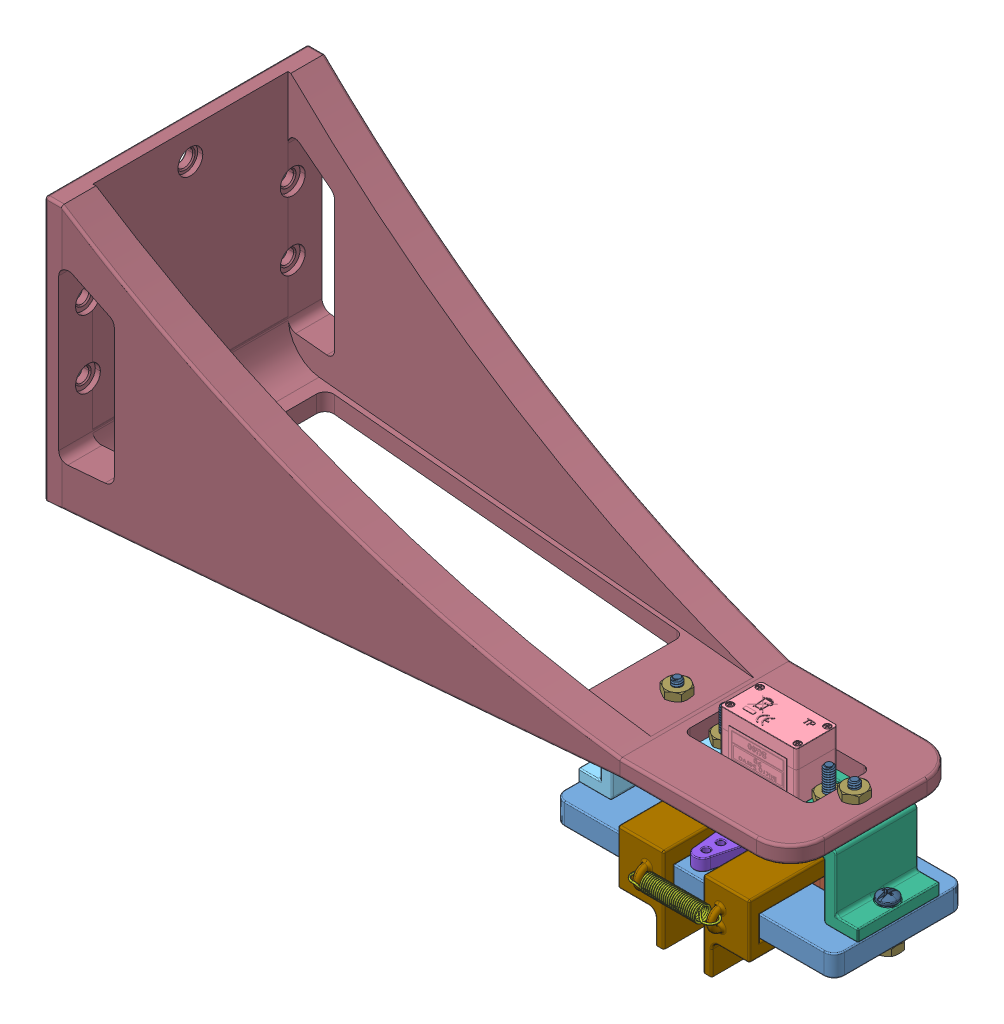
SolidWorks assembly Gripper_arm_assembly (1), configuration Default. Lengths in mm.
Overall size (212.31 117.38 77.37).
29 component instances, 13 part files, 0 mates.
Components (placement in the parent):
- Gripper_arm_assembly (1).STEP-1: Gripper_arm_assembly (1).STEP [Default] at origin size (212.31 117.38 77.37)
  - Plate.STEP-1: Plate.STEP [Default] at (-88.1203 -21.4219 2.3203) size (82 6.35 38)
  - ptfe_sleeve_bearing_6377K49.STEP-1: ptfe_sleeve_bearing_6377K49.STEP [Default] at (-73.4759 -18.2469 2.3203) x (1 0 0) z (0 -1 0) size (6.38 6.38 6.35)
  - ptfe_sleeve_bearing_6377K49.STEP-2: ptfe_sleeve_bearing_6377K49.STEP [Default] at (-102.0124 -18.2469 2.3203) x (0.999223 0 -0.039418) z (0 -1 0) size (6.38 6.38 6.35)
  - Shoulder Screw_90298A204.STEP-1: Shoulder Screw_90298A204.STEP [Default] at (-73.4759 -9.6469 2.3203) x (0.859262 0 0.511536) z (0 1 0) size (6.35 6.35 16.68)
  - Shoulder Screw_90298A204.STEP-2: Shoulder Screw_90298A204.STEP [Default] at (-102.0124 -9.6469 2.3203) x (0.259294 0 -0.965798) z (0 1 0) size (6.35 6.35 16.68)
  - Micro Feedback Servo_Pe_a.STEP-1: Micro Feedback Servo_Pe_a.STEP [Default] at (-82.647 8.3281 2.0203) x (1 0 0) z (0 0 -1) size (32.1 29.95 12.4)
  - left_bracket.STEP-1: left_bracket.STEP [Default] at (-116.2258 -5.2691 14.3203) x (-1 0 0) z (0 0 -1) size (41 20 24.01)
  - right_bracket.STEP-1: right_bracket.STEP [Default] at (-60.0149 -5.2691 -9.6797) size (30.25 20 24.01)
  - tension_spring_9433K38.STEP-1: tension_spring_9433K38.STEP [Default] at (-87.8838 -18.0406 -22.3607) x (1 0 0) z (0 1 0) size (25.45 4.86 5.05)
  - servo_horn.STEP-1: servo_horn.STEP [Default] at (-87.797 -7.8719 2.0203) x (0.076517 0 -0.997068) z (-0.997068 0 -0.076517) size (37 6.51 11)
  - gripper.STEP-1: gripper.STEP [Default] at (-79.8806 -26.0484 -20.1797) size (13.5 24.85 52.31)
  - gripper.STEP-2: gripper.STEP [Default] at (-95.6077 -26.0484 24.8203) x (-1 0 0) z (0 0 -1) size (13.5 24.85 52.31)
  - tension_spring_9433K38.STEP-2: tension_spring_9433K38.STEP [Default] at (-87.9272 -17.5634 27.1548) x (-1 0 0) z (0 1 0) size (25.45 4.86 5.05)
  - 90604A554_PAN HEAD COMBINATION PHILLIPSSLOTTED SCREWS_90604A554.STEP-1: 90604A554_PAN HEAD COMBINATION PHILLIPSSLOTTED SCREWS_90604A554.STEP [Default] at (-97.8703 14.1281 2.3203) x (0 0 -1) z (0 -1 0) size (5.56 5.56 14.68)
  - 90604A554_PAN HEAD COMBINATION PHILLIPSSLOTTED SCREWS_90604A554.STEP-2: 90604A554_PAN HEAD COMBINATION PHILLIPSSLOTTED SCREWS_90604A554.STEP [Default] at (-125.8703 -24.2719 2.3203) x (0 0 -1) z (0 1 0) size (5.56 5.56 14.68)
  - 90604A554_PAN HEAD COMBINATION PHILLIPSSLOTTED SCREWS_90604A554.STEP-3: 90604A554_PAN HEAD COMBINATION PHILLIPSSLOTTED SCREWS_90604A554.STEP [Default] at (-50.3703 -24.2719 2.3203) x (0 0 1) z (0 1 0) size (5.56 5.56 14.68)
  - 90604A554_PAN HEAD COMBINATION PHILLIPSSLOTTED SCREWS_90604A554.STEP-4: 90604A554_PAN HEAD COMBINATION PHILLIPSSLOTTED SCREWS_90604A554.STEP [Default] at (-67.6203 14.1281 2.3203) x (0 0 1) z (0 -1 0) size (5.56 5.56 14.68)
  - 91831A005_TYPE 18-8 STAINLESS STL NYLON-INSERT LOCKNUT_91831A005.STEP-1: 91831A005_TYPE 18-8 STAINLESS STL NYLON-INSERT LOCKNUT_91831A005.STEP [Default] at (-73.4759 -23.6719 2.3203) x (0.328008 0 -0.944675) z (-0.944675 0 -0.328008) size (6.37 3.58 7.35)
  - 91831A005_TYPE 18-8 STAINLESS STL NYLON-INSERT LOCKNUT_91831A005.STEP-2: 91831A005_TYPE 18-8 STAINLESS STL NYLON-INSERT LOCKNUT_91831A005.STEP [Default] at (-102.0124 -23.6719 2.3203) x (-0.99793 0 -0.064308) z (-0.064308 0 0.99793) size (6.37 3.58 7.35)
  - 91841A005_TYPE 18-8 STAINLESS STEEL HEX NUT_91841A005.STEP-1: 91841A005_TYPE 18-8 STAINLESS STEEL HEX NUT_91841A005.STEP [Default] at (-50.3703 -22.6125 2.3203) x (0.999219 0 0.039522) z (-0.039522 0 0.999219) size (7.34 2.4 7.35)
  - 91841A005_TYPE 18-8 STAINLESS STEEL HEX NUT_91841A005.STEP-2: 91841A005_TYPE 18-8 STAINLESS STEEL HEX NUT_91841A005.STEP [Default] at (-125.8703 -22.6125 2.3203) x (0.981662 0 0.19063) z (-0.19063 0 0.981662) size (7.34 2.4 7.35)
  - 91841A005_TYPE 18-8 STAINLESS STEEL HEX NUT_91841A005.STEP-3: 91841A005_TYPE 18-8 STAINLESS STEEL HEX NUT_91841A005.STEP [Default] at (-67.6203 6.1187 2.3203) x (0.999956 0 0.009417) z (-0.009417 0 0.999956) size (7.34 2.4 7.35)
  - 91841A005_TYPE 18-8 STAINLESS STEEL HEX NUT_91841A005.STEP-4: 91841A005_TYPE 18-8 STAINLESS STEEL HEX NUT_91841A005.STEP [Default] at (-97.8703 6.1187 2.3203) x (0.99945 0 0.033169) z (-0.033169 0 0.99945) size (7.34 2.4 7.35)
  - Arm_reduced.STEP-1: Arm_reduced.STEP [Default] at (-253.8703 43.5031 2.3203) x (0 0 1) z (1 0 0) size (77.37 77.78 205)
  - 91841A005_TYPE 18-8 STAINLESS STEEL HEX NUT_91841A005.STEP-5: 91841A005_TYPE 18-8 STAINLESS STEEL HEX NUT_91841A005.STEP [Default] at (-112.1203 11.1187 2.3203) size (7.34 2.4 7.35)
  - 91841A005_TYPE 18-8 STAINLESS STEEL HEX NUT_91841A005.STEP-6: 91841A005_TYPE 18-8 STAINLESS STEEL HEX NUT_91841A005.STEP [Default] at (-60.1203 11.1187 2.3203) size (7.34 2.4 7.35)
  - 90604A554_PAN HEAD COMBINATION PHILLIPSSLOTTED SCREWS_90604A554.STEP-5: 90604A554_PAN HEAD COMBINATION PHILLIPSSLOTTED SCREWS_90604A554.STEP [Default] at (-112.1203 14.1281 2.3203) x (-0.643739 0 0.765245) z (0 -1 0) size (5.56 5.56 14.68)
  - 90604A554_PAN HEAD COMBINATION PHILLIPSSLOTTED SCREWS_90604A554.STEP-6: 90604A554_PAN HEAD COMBINATION PHILLIPSSLOTTED SCREWS_90604A554.STEP [Default] at (-60.1203 14.1281 2.3203) x (-0.027091 0 -0.999633) z (0 -1 0) size (5.56 5.56 14.68)
